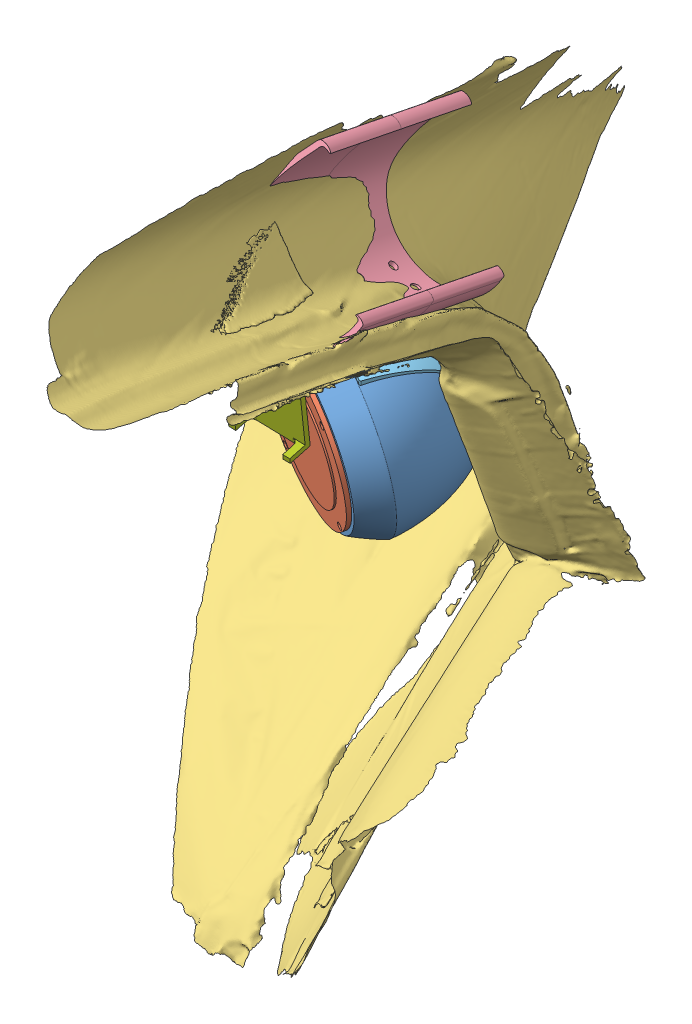
SolidWorks assembly 汽车音箱组装.SLDA-万向SM, configuration Default. Lengths in mm.
Overall size (276.78 370.21 467.74).
8 component instances, 7 part files, 11 mates.
Components (placement in the parent):
- 汽车音箱-1: 汽车音箱 [Default] at (-106.3954 93.1549 77.9619) x (-0.113502 -0.967067 -0.227814) z (0.918563 -0.189523 0.346875) size (109.81 81.39 109.81)
- 莞音3寸圆-1: 莞音3寸圆 [Default] at (-107.3419 92.7302 80.2364) x (0.65206 -0.746597 0.131947) z (0.656855 0.643218 0.393461) size (89 52 89)
- focus_a-1: focus_a [Default] at (-114.0656 67.5174 400.1558) size (276.78 370.21 467.74)
- focus_a_a_clear-2-圆形接口-1: focus_a_a_clear-2-圆形接口 [默认] at (-132.0054 33.9996 301.115) size (76.57 112.34 74.02)
- 音箱支架-上-万向-1: 音箱支架-上-万向 [默认] at (-103.9651 95.7274 68.4142) x (0.201157 0.971835 0.122773) z (-0.914469 0.231235 -0.33208) size (53.4 68.23 66.01)
- 音箱支架-上-万向-盖子-1: 音箱支架-上-万向-盖子 [默认] at (-102.9971 154.5384 38.6925) x (0.948308 -0.31711 -0.012398) z (0.10389 0.273291 0.956305) size (15 5 36)
- focus_a_a_clear-2-圆形接口-2: focus_a_a_clear-2-圆形接口 [默认] at (-126.8109 47.6641 348.9302) size (76.57 112.34 74.02)
- 手机固定-1: 手机固定 [默认] at (-60.09 175.3547 130.8914) x (-0.993456 0.092525 0.066968) z (-0.104093 -0.97478 -0.197406) size (35 42.9 53.95)
Mates (geometry in assembly coordinates):
- Concentric1: concentric anti-aligned: cylinder of 汽车音箱-1 through (-105.2595 93.6646 75.2324) axis (-0.378627 -0.16989 0.909823) radius 36.5; cone of 莞音3寸圆-1 through (-106.3954 93.1549 77.9619) axis (0.378627 0.16989 -0.909823)
- Coincident1: coincident anti-aligned: plane of 汽车音箱-1 through (-106.3954 93.1549 77.9619) normal (-0.378627 -0.16989 0.909823); plane of 莞音3寸圆-1 through (-106.3954 93.1549 77.9619) normal (0.378627 0.16989 -0.909823)
- 同心1: concentric: sphere of focus_a_a_clear-2-圆形接口-1; sphere of 音箱支架-上-万向-1
- 锁定1: lock: unknown of 汽车音箱-1; unknown of 音箱支架-上-万向-1
- 距离1: distance = 0 mm anti-aligned: plane of focus_a_a_clear-2-圆形接口-1 through (-89.2272 170.3776 84.9547) normal (-0.299865 -0.908159 0.292109); plane of 音箱支架-上-万向-盖子-1 through (-101.4977 159.0792 37.2319) normal (0.299865 0.908159 -0.292109)
- 同心2: concentric aligned: cylinder of focus_a_a_clear-2-圆形接口-1 through (-53.2472 278.166 36.6483) axis (-0.299865 -0.908159 0.292109) radius 1.65; cylinder of 音箱支架-上-万向-盖子-1 through (-90.0673 166.6541 72.516) axis (-0.299865 -0.908159 0.292109) radius 1.65
- 同心3: concentric aligned: cylinder of focus_a_a_clear-2-圆形接口-1 through (-55.7406 271.607 13.697) axis (-0.299865 -0.908159 0.292109) radius 1.65; cylinder of 音箱支架-上-万向-盖子-1 through (-92.5607 160.0951 49.5647) axis (-0.299865 -0.908159 0.292109) radius 1.65
- 重合1: coincident anti-aligned: plane of focus_a_a_clear-2-圆形接口-1 through (-149.1472 -11.0935 143.3247) normal (0.10389 0.273291 0.956305); plane of focus_a_a_clear-2-圆形接口-2 through (-149.1472 -11.0935 143.3247) normal (-0.10389 -0.273291 -0.956305)
- 同心4: concentric aligned: circle of focus_a_a_clear-2-圆形接口-1; circle of focus_a_a_clear-2-圆形接口-2
- 重合3: coincident aligned: line of focus_a_a_clear-2-圆形接口-1 through (-79.9272 261.9415 57.7773) axis (-0.10389 -0.273291 -0.956305); line of focus_a_a_clear-2-圆形接口-2 through (-74.7327 275.6061 105.5926) axis (-0.10389 -0.273291 -0.956305)
- 同心6: concentric: sphere of focus_a_a_clear-2-圆形接口-2; sphere of 手机固定-1
